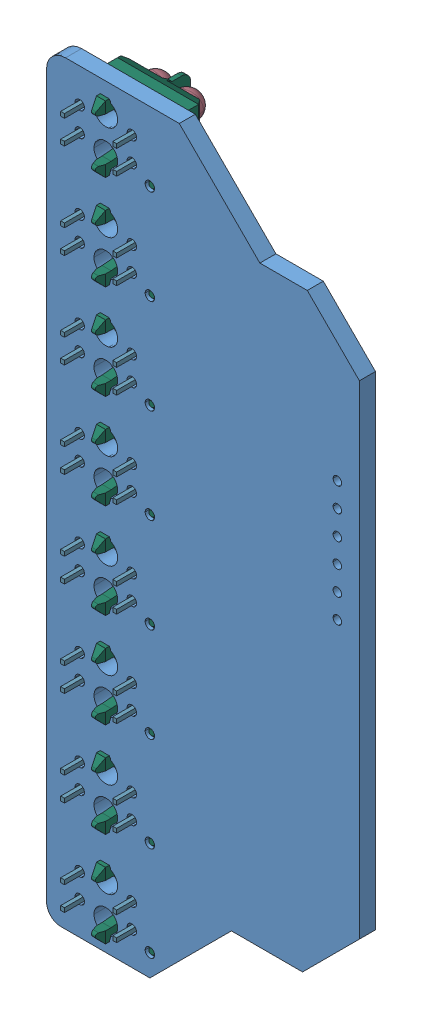
SolidWorks assembly Linelance_PCB v1.1, configuration По умолчанию. Lengths in mm. (continued)
Components (placement in the parent): (continued)
- Linelance_PCB v1.1.step-1: Linelance_PCB v1.1.step [По умолчанию] at origin size (33 79.6 10.52) (continued)
  - Linelance_PCB v1.1.step.step-1: Linelance_PCB v1.1.step.step [По умолчанию] at origin size (33 79.6 10.52) (continued)
    - R8.step.step-1: R8.step.step [По умолчанию] at origin size (0.8 1.6 0.5) (continued)
      - 5770190160.step-6.step-1: 5770190160.step-6.step [По умолчанию] at (4.2 69.8 -1.692) x (0 -1 0) z (0 0 -1) size (1.6 0.8 0.5)
        - Terminal-2.step-12.step-1: Terminal-2.step-12.step [По умолчанию] at (-0.8 -0.4 0) size (0.3 0.8 0.5)
          - Open_CASCADE_STEP_translator_6.8_7.2.1-6.step.step-1: Open_CASCADE_STEP_translator_6.8_7.2.1-6.step.step [По умолчанию] at origin size (0.3 0.8 0.5)
        - Terminal-2.step-13.step-1: Terminal-2.step-13.step [По умолчанию] at (0.8 0.4 0) x (-1 0 0) z (0 0 1) size (0.3 0.8 0.5)
          - Open_CASCADE_STEP_translator_6.8_7.2.1-6.step.step-1: Open_CASCADE_STEP_translator_6.8_7.2.1-6.step.step [По умолчанию] at origin size (0.3 0.8 0.5)
        - Mid_Body-7.step.step-1: Mid_Body-7.step.step [По умолчанию] at (-0.8 -0.4 0) size (1.5 0.8 0.4)
        - Mark-8.step.step-1: Mark-8.step.step [По умолчанию] at (-0.5 -0.4 0.45) size (1 0.8 0.05)
    - R7.step.step-1: R7.step.step [По умолчанию] at origin size (1.6 0.8 0.5)
      - 5770196880.step-1.step-1: 5770196880.step-1.step [По умолчанию] at (20.1975 53.1275 -1.692) x (-1 0 0) z (0 0 -1) size (1.6 0.8 0.5)
        - Terminal.step-2.step-1: Terminal.step-2.step [По умолчанию] at (-0.8 -0.4 0) size (0.3 0.8 0.5)
          - Open_CASCADE_STEP_translator_6.8_7.2.1.step.step-1: Open_CASCADE_STEP_translator_6.8_7.2.1.step.step [По умолчанию] at origin size (0.3 0.8 0.5)
        - Terminal.step-3.step-1: Terminal.step-3.step [По умолчанию] at (0.8 0.4 0) x (-1 0 0) z (0 0 1) size (0.3 0.8 0.5)
          - Open_CASCADE_STEP_translator_6.8_7.2.1.step.step-1: Open_CASCADE_STEP_translator_6.8_7.2.1.step.step [По умолчанию] at origin size (0.3 0.8 0.5)
        - Mid_Body.step.step-1: Mid_Body.step.step [По умолчанию] at (-0.8 -0.4 0) size (1.5 0.8 0.4)
        - Mark.step.step-1: Mark.step.step [По умолчанию] at (-0.5 -0.4 0.45) size (1 0.8 0.05)
    - R6.step.step-1: R6.step.step [По умолчанию] at origin size (1.6 0.8 0.5)
      - 5770190480.step.step-1: 5770190480.step.step [По умолчанию] at (20.9975 51.7275 -1.692) x (1 0 0) z (0 0 -1) size (1.6 0.8 0.5)
        - Terminal-3.step.step-1: Terminal-3.step.step [По умолчанию] at (-0.8 -0.4 0) size (0.3 0.8 0.5)
          - Open_CASCADE_STEP_translator_6.8_7.2.1-9.step.step-1: Open_CASCADE_STEP_translator_6.8_7.2.1-9.step.step [По умолчанию] at origin size (0.3 0.8 0.5)
        - Terminal-3.step-1.step-1: Terminal-3.step-1.step [По умолчанию] at (0.8 0.4 0) x (-1 0 0) z (0 0 1) size (0.3 0.8 0.5)
          - Open_CASCADE_STEP_translator_6.8_7.2.1-9.step.step-1: Open_CASCADE_STEP_translator_6.8_7.2.1-9.step.step [По умолчанию] at origin size (0.3 0.8 0.5)
        - Mid_Body-10.step.step-1: Mid_Body-10.step.step [По умолчанию] at (-0.8 -0.4 0) size (1.5 0.8 0.4)
        - Mark-11.step.step-1: Mark-11.step.step [По умолчанию] at (-0.5 -0.4 0.45) size (1 0.8 0.05)
    - R3.step.step-1: R3.step.step [По умолчанию] at origin size (0.8 1.6 0.5)
      - 5770190160.step-7.step-1: 5770190160.step-7.step [По умолчанию] at (18.5 26.9 -1.692) x (0 -1 0) z (0 0 -1) size (1.6 0.8 0.5)
        - Terminal-2.step-14.step-1: Terminal-2.step-14.step [По умолчанию] at (-0.8 -0.4 0) size (0.3 0.8 0.5)
          - Open_CASCADE_STEP_translator_6.8_7.2.1-6.step.step-1: Open_CASCADE_STEP_translator_6.8_7.2.1-6.step.step [По умолчанию] at origin size (0.3 0.8 0.5)
        - Terminal-2.step-15.step-1: Terminal-2.step-15.step [По умолчанию] at (0.8 0.4 0) x (-1 0 0) z (0 0 1) size (0.3 0.8 0.5)
          - Open_CASCADE_STEP_translator_6.8_7.2.1-6.step.step-1: Open_CASCADE_STEP_translator_6.8_7.2.1-6.step.step [По умолчанию] at origin size (0.3 0.8 0.5)
        - Mid_Body-7.step.step-1: Mid_Body-7.step.step [По умолчанию] at (-0.8 -0.4 0) size (1.5 0.8 0.4)
        - Mark-8.step.step-1: Mark-8.step.step [По умолчанию] at (-0.5 -0.4 0.45) size (1 0.8 0.05)
    - R2.step.step-1: R2.step.step [По умолчанию] at origin size (1.6 0.8 0.5)
      - 5770190480.step-1.step-1: 5770190480.step-1.step [По умолчанию] at (26.5 22.6 -1.692) x (1 0 0) z (0 0 -1) size (1.6 0.8 0.5)
        - Terminal-3.step-2.step-1: Terminal-3.step-2.step [По умолчанию] at (-0.8 -0.4 0) size (0.3 0.8 0.5)
          - Open_CASCADE_STEP_translator_6.8_7.2.1-9.step.step-1: Open_CASCADE_STEP_translator_6.8_7.2.1-9.step.step [По умолчанию] at origin size (0.3 0.8 0.5)
        - Terminal-3.step-3.step-1: Terminal-3.step-3.step [По умолчанию] at (0.8 0.4 0) x (-1 0 0) z (0 0 1) size (0.3 0.8 0.5)
          - Open_CASCADE_STEP_translator_6.8_7.2.1-9.step.step-1: Open_CASCADE_STEP_translator_6.8_7.2.1-9.step.step [По умолчанию] at origin size (0.3 0.8 0.5)
        - Mid_Body-10.step.step-1: Mid_Body-10.step.step [По умолчанию] at (-0.8 -0.4 0) size (1.5 0.8 0.4)
        - Mark-11.step.step-1: Mark-11.step.step [По умолчанию] at (-0.5 -0.4 0.45) size (1 0.8 0.05)
    - R5.step.step-1: R5.step.step [По умолчанию] at origin size (1.6 0.8 0.5)
      - 5770190480.step-2.step-1: 5770190480.step-2.step [По умолчанию] at (30.3 39.9 -1.692) x (1 0 0) z (0 0 -1) size (1.6 0.8 0.5)
        - Terminal-3.step-4.step-1: Terminal-3.step-4.step [По умолчанию] at (-0.8 -0.4 0) size (0.3 0.8 0.5)
          - Open_CASCADE_STEP_translator_6.8_7.2.1-9.step.step-1: Open_CASCADE_STEP_translator_6.8_7.2.1-9.step.step [По умолчанию] at origin size (0.3 0.8 0.5)
        - Terminal-3.step-5.step-1: Terminal-3.step-5.step [По умолчанию] at (0.8 0.4 0) x (-1 0 0) z (0 0 1) size (0.3 0.8 0.5)
          - Open_CASCADE_STEP_translator_6.8_7.2.1-9.step.step-1: Open_CASCADE_STEP_translator_6.8_7.2.1-9.step.step [По умолчанию] at origin size (0.3 0.8 0.5)
        - Mid_Body-10.step.step-1: Mid_Body-10.step.step [По умолчанию] at (-0.8 -0.4 0) size (1.5 0.8 0.4)
        - Mark-11.step.step-1: Mark-11.step.step [По умолчанию] at (-0.5 -0.4 0.45) size (1 0.8 0.05)
    - R4.step.step-1: R4.step.step [По умолчанию] at origin size (1.6 0.8 0.5)
      - 5770190480.step-3.step-1: 5770190480.step-3.step [По умолчанию] at (30.3 38.5 -1.692) x (1 0 0) z (0 0 -1) size (1.6 0.8 0.5)
        - Terminal-3.step-6.step-1: Terminal-3.step-6.step [По умолчанию] at (-0.8 -0.4 0) size (0.3 0.8 0.5)
          - Open_CASCADE_STEP_translator_6.8_7.2.1-9.step.step-1: Open_CASCADE_STEP_translator_6.8_7.2.1-9.step.step [По умолчанию] at origin size (0.3 0.8 0.5)
        - Terminal-3.step-7.step-1: Terminal-3.step-7.step [По умолчанию] at (0.8 0.4 0) x (-1 0 0) z (0 0 1) size (0.3 0.8 0.5)
          - Open_CASCADE_STEP_translator_6.8_7.2.1-9.step.step-1: Open_CASCADE_STEP_translator_6.8_7.2.1-9.step.step [По умолчанию] at origin size (0.3 0.8 0.5)
        - Mid_Body-10.step.step-1: Mid_Body-10.step.step [По умолчанию] at (-0.8 -0.4 0) size (1.5 0.8 0.4)
        - Mark-11.step.step-1: Mark-11.step.step [По умолчанию] at (-0.5 -0.4 0.45) size (1 0.8 0.05)
    - L4.step.step-1: L4.step.step [По умолчанию] at origin size (3.2 1.6 1.8)
      - 5770190080.step.step-1: 5770190080.step.step [По умолчанию] at (19.2675 55.0275 -1.692) x (-1 0 0) z (0 0 -1) size (3.2 1.6 1.8)
        - Terminal-4.step.step-1: Terminal-4.step.step [По умолчанию] at (-1.6 -0.8 0) size (3.2 1.6 1.8)
          - Open_CASCADE_STEP_translator_6.8_9.1.1.step.step-1: Open_CASCADE_STEP_translator_6.8_9.1.1.step.step [По умолчанию] at origin size (0.7 1.6 1.8)
          - Open_CASCADE_STEP_translator_6.8_9.1.2.step.step-1: Open_CASCADE_STEP_translator_6.8_9.1.2.step.step [По умолчанию] at origin size (0.7 1.6 1.8)
        - Mid_Body-12.step.step-1: Mid_Body-12.step.step [По умолчанию] at (-1.6 -0.8 0) size (1.8 1.6 1.8)
          - Open_CASCADE_STEP_translator_6.8_9.2.1.step.step-1: Open_CASCADE_STEP_translator_6.8_9.2.1.step.step [По умолчанию] at origin size (1.8 1.6 1.8)
    - L3.step.step-1: L3.step.step [По умолчанию] at origin size (1.6 3.2 1.8)
      - 5770196320.step.step-1: 5770196320.step.step [По умолчанию] at (19 40.5 -1.692) x (0 -1 0) z (0 0 -1) size (3.2 1.6 1.8)
        - Terminal-5.step.step-1: Terminal-5.step.step [По умолчанию] at (-1.6 -0.8 0) size (3.2 1.6 1.8)
          - Open_CASCADE_STEP_translator_6.8_9.1.1-13.step.step-1: Open_CASCADE_STEP_translator_6.8_9.1.1-13.step.step [По умолчанию] at origin size (0.7 1.6 1.8)
          - Open_CASCADE_STEP_translator_6.8_9.1.2-14.step.step-1: Open_CASCADE_STEP_translator_6.8_9.1.2-14.step.step [По умолчанию] at origin size (0.7 1.6 1.8)
        - Mid_Body-1.step.step-1: Mid_Body-1.step.step [По умолчанию] at (-1.6 -0.8 0) size (1.8 1.6 1.8)
          - Open_CASCADE_STEP_translator_6.8_9.2.1-15.step.step-1: Open_CASCADE_STEP_translator_6.8_9.2.1-15.step.step [По умолчанию] at origin size (1.8 1.6 1.8)
    - L2.step.step-1: L2.step.step [По умолчанию] at origin size (1.6 3.2 1.8)
      - 5770196320.step-1.step-1: 5770196320.step-1.step [По умолчанию] at (21.2975 44.5275 -1.692) x (0 -1 0) z (0 0 -1) size (3.2 1.6 1.8)
        - Terminal-5.step-1.step-1: Terminal-5.step-1.step [По умолчанию] at (-1.6 -0.8 0) size (3.2 1.6 1.8)
          - Open_CASCADE_STEP_translator_6.8_9.1.1-13.step.step-1: Open_CASCADE_STEP_translator_6.8_9.1.1-13.step.step [По умолчанию] at origin size (0.7 1.6 1.8)
          - Open_CASCADE_STEP_translator_6.8_9.1.2-14.step.step-1: Open_CASCADE_STEP_translator_6.8_9.1.2-14.step.step [По умолчанию] at origin size (0.7 1.6 1.8)
        - Mid_Body-1.step-1.step-1: Mid_Body-1.step-1.step [По умолчанию] at (-1.6 -0.8 0) size (1.8 1.6 1.8)
          - Open_CASCADE_STEP_translator_6.8_9.2.1-15.step.step-1: Open_CASCADE_STEP_translator_6.8_9.2.1-15.step.step [По умолчанию] at origin size (1.8 1.6 1.8)
    - L1.step.step-1: L1.step.step [По умолчанию] at origin size (3.2 1.6 1.8)
      - 5770190080.step-1.step-1: 5770190080.step-1.step [По умолчанию] at (24.1 57.3 -1.692) x (-1 0 0) z (0 0 -1) size (3.2 1.6 1.8)
        - Terminal-4.step-1.step-1: Terminal-4.step-1.step [По умолчанию] at (-1.6 -0.8 0) size (3.2 1.6 1.8)
          - Open_CASCADE_STEP_translator_6.8_9.1.1.step.step-1: Open_CASCADE_STEP_translator_6.8_9.1.1.step.step [По умолчанию] at origin size (0.7 1.6 1.8)
          - Open_CASCADE_STEP_translator_6.8_9.1.2.step.step-1: Open_CASCADE_STEP_translator_6.8_9.1.2.step.step [По умолчанию] at origin size (0.7 1.6 1.8)
        - Mid_Body-12.step-1.step-1: Mid_Body-12.step-1.step [По умолчанию] at (-1.6 -0.8 0) size (1.8 1.6 1.8)
          - Open_CASCADE_STEP_translator_6.8_9.2.1.step.step-1: Open_CASCADE_STEP_translator_6.8_9.2.1.step.step [По умолчанию] at origin size (1.8 1.6 1.8)
    - D1.step.step-1: D1.step.step [По умолчанию] at origin size (1.7 0.9 0.7)
      - SOD523.step.step-1: SOD523.step.step [По умолчанию] at (30.4001 58.3999 -1.692) x (1 0 0) z (0 0 -1) size (1.7 0.9 0.7)
    - C21.step.step-1: C21.step.step [По умолчанию] at origin size (0.8 1.6 0.5)
      - 5899457520.step-1.step-1: 5899457520.step-1.step [По умолчанию] at (17.9975 52.3525 -2.192) size (0.8 1 0.5)
        - Extruded-1.step.step-1: Extruded-1.step.step [По умолчанию] at origin size (0.8 1 0.5)
      - 5899457200.step-2.step-1: 5899457200.step-2.step [По умолчанию] at (17.9975 53.0025 -2.192) size (0.8 0.3 0.5)
        - Extruded-2.step.step-1: Extruded-2.step.step [По умолчанию] at origin size (0.8 0.3 0.5)
      - 5899457200.step-3.step-1: 5899457200.step-3.step [По умолчанию] at (17.9975 51.7025 -2.192) size (0.8 0.3 0.5)
        - Extruded-2.step.step-1: Extruded-2.step.step [По умолчанию] at origin size (0.8 0.3 0.5)
    - C20.step.step-1: C20.step.step [По умолчанию] at origin size (0.8 1.6 0.5)
      - 5899457200.step-4.step-1: 5899457200.step-4.step [По умолчанию] at (17.9975 49.9775 -2.192) size (0.8 0.3 0.5)
        - Extruded-2.step.step-1: Extruded-2.step.step [По умолчанию] at origin size (0.8 0.3 0.5)
      - 5899457200.step-5.step-1: 5899457200.step-5.step [По умолчанию] at (17.9975 48.6775 -2.192) size (0.8 0.3 0.5)
        - Extruded-2.step.step-1: Extruded-2.step.step [По умолчанию] at origin size (0.8 0.3 0.5)
      - 5899457520.step-2.step-1: 5899457520.step-2.step [По умолчанию] at (17.9975 49.3275 -2.192) size (0.8 1 0.5)
        - Extruded-1.step.step-1: Extruded-1.step.step [По умолчанию] at origin size (0.8 1 0.5)
    - C14.step.step-1: C14.step.step [По умолчанию] at origin size (1.6 0.8 0.5)
      - 5899458880.step-4.step-1: 5899458880.step-4.step [По умолчанию] at (18.6 36.1 -2.192) size (1 0.8 0.5)
        - Extruded.step.step-1: Extruded.step.step [По умолчанию] at origin size (1 0.8 0.5)
      - 5899458400.step-8.step-1: 5899458400.step-8.step [По умолчанию] at (19.25 36.1 -2.192) size (0.3 0.8 0.5)
        - Extruded-0.step.step-1: Extruded-0.step.step [По умолчанию] at origin size (0.3 0.8 0.5)
      - 5899458400.step-9.step-1: 5899458400.step-9.step [По умолчанию] at (17.95 36.1 -2.192) size (0.3 0.8 0.5)
        - Extruded-0.step.step-1: Extruded-0.step.step [По умолчанию] at origin size (0.3 0.8 0.5)
    - C13.step.step-1: C13.step.step [По умолчанию] at origin size (1.6 0.8 0.5)
      - 5899458880.step-5.step-1: 5899458880.step-5.step [По умолчанию] at (18.6 37.4 -2.192) size (1 0.8 0.5)
        - Extruded.step.step-1: Extruded.step.step [По умолчанию] at origin size (1 0.8 0.5)
      - 5899458400.step-10.step-1: 5899458400.step-10.step [По умолчанию] at (19.25 37.4 -2.192) size (0.3 0.8 0.5)
        - Extruded-0.step.step-1: Extruded-0.step.step [По умолчанию] at origin size (0.3 0.8 0.5)
      - 5899458400.step-11.step-1: 5899458400.step-11.step [По умолчанию] at (17.95 37.4 -2.192) size (0.3 0.8 0.5)
        - Extruded-0.step.step-1: Extruded-0.step.step [По умолчанию] at origin size (0.3 0.8 0.5)
    - C9.step.step-1: C9.step.step [По умолчанию] at origin size (0.8 1.6 0.5)
      - 5899457520.step-3.step-1: 5899457520.step-3.step [По умолчанию] at (23.2 43.7 -2.192) size (0.8 1 0.5)
        - Extruded-1.step.step-1: Extruded-1.step.step [По умолчанию] at origin size (0.8 1 0.5)
      - 5899457200.step-6.step-1: 5899457200.step-6.step [По умолчанию] at (23.2 43.05 -2.192) size (0.8 0.3 0.5)
        - Extruded-2.step.step-1: Extruded-2.step.step [По умолчанию] at origin size (0.8 0.3 0.5)
      - 5899457200.step-7.step-1: 5899457200.step-7.step [По умолчанию] at (23.2 44.35 -2.192) size (0.8 0.3 0.5)
        - Extruded-2.step.step-1: Extruded-2.step.step [По умолчанию] at origin size (0.8 0.3 0.5)
    - C10.step.step-1: C10.step.step [По умолчанию] at origin size (0.8 1.6 0.5)
      - 5899457520.step-4.step-1: 5899457520.step-4.step [По умолчанию] at (24.7 43.7 -2.192) size (0.8 1 0.5)
        - Extruded-1.step.step-1: Extruded-1.step.step [По умолчанию] at origin size (0.8 1 0.5)
      - 5899457200.step-8.step-1: 5899457200.step-8.step [По умолчанию] at (24.7 43.05 -2.192) size (0.8 0.3 0.5)
        - Extruded-2.step.step-1: Extruded-2.step.step [По умолчанию] at origin size (0.8 0.3 0.5)
      - 5899457200.step-9.step-1: 5899457200.step-9.step [По умолчанию] at (24.7 44.35 -2.192) size (0.8 0.3 0.5)
        - Extruded-2.step.step-1: Extruded-2.step.step [По умолчанию] at origin size (0.8 0.3 0.5)
    - C12.step.step-1: C12.step.step [По умолчанию] at origin size (0.8 1.6 0.5)
      - 5899457520.step-5.step-1: 5899457520.step-5.step [По умолчанию] at (27.6968 43.7 -2.192) size (0.8 1 0.5)
        - Extruded-1.step.step-1: Extruded-1.step.step [По умолчанию] at origin size (0.8 1 0.5)
      - 5899457200.step-10.step-1: 5899457200.step-10.step [По умолчанию] at (27.6968 43.05 -2.192) size (0.8 0.3 0.5)
        - Extruded-2.step.step-1: Extruded-2.step.step [По умолчанию] at origin size (0.8 0.3 0.5)
      - 5899457200.step-11.step-1: 5899457200.step-11.step [По умолчанию] at (27.6968 44.35 -2.192) size (0.8 0.3 0.5)
        - Extruded-2.step.step-1: Extruded-2.step.step [По умолчанию] at origin size (0.8 0.3 0.5)
    - C19.step.step-1: C19.step.step [По умолчанию] at origin size (0.8 1.6 0.5)
      - 5899457520.step-6.step-1: 5899457520.step-6.step [По умолчанию] at (20 25.7 -2.192) size (0.8 1 0.5)
        - Extruded-1.step.step-1: Extruded-1.step.step [По умолчанию] at origin size (0.8 1 0.5)
      - 5899457200.step-12.step-1: 5899457200.step-12.step [По умолчанию] at (20 26.35 -2.192) size (0.8 0.3 0.5)
        - Extruded-2.step.step-1: Extruded-2.step.step [По умолчанию] at origin size (0.8 0.3 0.5)
      - 5899457200.step-13.step-1: 5899457200.step-13.step [По умолчанию] at (20 25.05 -2.192) size (0.8 0.3 0.5)
        - Extruded-2.step.step-1: Extruded-2.step.step [По умолчанию] at origin size (0.8 0.3 0.5)
    - C18.step.step-1: C18.step.step [По умолчанию] at origin size (1.6 0.8 0.5)
      - 5899458880.step-6.step-1: 5899458880.step-6.step [По умолчанию] at (25.3 32.2 -2.192) size (1 0.8 0.5)
        - Extruded.step.step-1: Extruded.step.step [По умолчанию] at origin size (1 0.8 0.5)
      - 5899458400.step-12.step-1: 5899458400.step-12.step [По умолчанию] at (25.95 32.2 -2.192) size (0.3 0.8 0.5)
        - Extruded-0.step.step-1: Extruded-0.step.step [По умолчанию] at origin size (0.3 0.8 0.5)
      - 5899458400.step-13.step-1: 5899458400.step-13.step [По умолчанию] at (24.65 32.2 -2.192) size (0.3 0.8 0.5)
        - Extruded-0.step.step-1: Extruded-0.step.step [По умолчанию] at origin size (0.3 0.8 0.5)
    - C17.step.step-1: C17.step.step [По умолчанию] at origin size (1.6 0.8 0.5)
      - 5899458880.step-7.step-1: 5899458880.step-7.step [По умолчанию] at (23.3 33.7 -2.192) size (1 0.8 0.5)
        - Extruded.step.step-1: Extruded.step.step [По умолчанию] at origin size (1 0.8 0.5)
      - 5899458400.step-14.step-1: 5899458400.step-14.step [По умолчанию] at (22.65 33.7 -2.192) size (0.3 0.8 0.5)
        - Extruded-0.step.step-1: Extruded-0.step.step [По умолчанию] at origin size (0.3 0.8 0.5)
      - 5899458400.step-15.step-1: 5899458400.step-15.step [По умолчанию] at (23.95 33.7 -2.192) size (0.3 0.8 0.5)
        - Extruded-0.step.step-1: Extruded-0.step.step [По умолчанию] at origin size (0.3 0.8 0.5)
    - C5.step.step-1: C5.step.step [По умолчанию] at origin size (0.8 1.6 0.5)
      - 5899457520.step-7.step-1: 5899457520.step-7.step [По умолчанию] at (27.7 46.7 -2.192) size (0.8 1 0.5)
        - Extruded-1.step.step-1: Extruded-1.step.step [По умолчанию] at origin size (0.8 1 0.5)
      - 5899457200.step-14.step-1: 5899457200.step-14.step [По умолчанию] at (27.7 47.35 -2.192) size (0.8 0.3 0.5)
        - Extruded-2.step.step-1: Extruded-2.step.step [По умолчанию] at origin size (0.8 0.3 0.5)
      - 5899457200.step-15.step-1: 5899457200.step-15.step [По умолчанию] at (27.7 46.05 -2.192) size (0.8 0.3 0.5)
        - Extruded-2.step.step-1: Extruded-2.step.step [По умолчанию] at origin size (0.8 0.3 0.5)
    - C8.step.step-1: C8.step.step [По умолчанию] at origin size (0.8 1.6 0.5)
      - 5899457520.step-8.step-1: 5899457520.step-8.step [По умолчанию] at (23.2 46.7 -2.192) size (0.8 1 0.5)
        - Extruded-1.step.step-1: Extruded-1.step.step [По умолчанию] at origin size (0.8 1 0.5)
      - 5899457200.step-16.step-1: 5899457200.step-16.step [По умолчанию] at (23.2 46.05 -2.192) size (0.8 0.3 0.5)
        - Extruded-2.step.step-1: Extruded-2.step.step [По умолчанию] at origin size (0.8 0.3 0.5)
      - 5899457200.step-17.step-1: 5899457200.step-17.step [По умолчанию] at (23.2 47.35 -2.192) size (0.8 0.3 0.5)
        - Extruded-2.step.step-1: Extruded-2.step.step [По умолчанию] at origin size (0.8 0.3 0.5)
    - C7.step.step-1: C7.step.step [По умолчанию] at origin size (0.8 1.6 0.5)
      - 5899457520.step-9.step-1: 5899457520.step-9.step [По умолчанию] at (24.7 46.7 -2.192) size (0.8 1 0.5)
        - Extruded-1.step.step-1: Extruded-1.step.step [По умолчанию] at origin size (0.8 1 0.5)
      - 5899457200.step-18.step-1: 5899457200.step-18.step [По умолчанию] at (24.7 46.05 -2.192) size (0.8 0.3 0.5)
        - Extruded-2.step.step-1: Extruded-2.step.step [По умолчанию] at origin size (0.8 0.3 0.5)
      - 5899457200.step-19.step-1: 5899457200.step-19.step [По умолчанию] at (24.7 47.35 -2.192) size (0.8 0.3 0.5)
        - Extruded-2.step.step-1: Extruded-2.step.step [По умолчанию] at origin size (0.8 0.3 0.5)
    - C6.step.step-1: C6.step.step [По умолчанию] at origin size (0.8 1.6 0.5)
      - 5899457520.step-10.step-1: 5899457520.step-10.step [По умолчанию] at (26.2 46.7 -2.192) size (0.8 1 0.5)
        - Extruded-1.step.step-1: Extruded-1.step.step [По умолчанию] at origin size (0.8 1 0.5)
      - 5899457200.step-20.step-1: 5899457200.step-20.step [По умолчанию] at (26.2 46.05 -2.192) size (0.8 0.3 0.5)
        - Extruded-2.step.step-1: Extruded-2.step.step [По умолчанию] at origin size (0.8 0.3 0.5)
      - 5899457200.step-21.step-1: 5899457200.step-21.step [По умолчанию] at (26.2 47.35 -2.192) size (0.8 0.3 0.5)
        - Extruded-2.step.step-1: Extruded-2.step.step [По умолчанию] at origin size (0.8 0.3 0.5)
    - C3.step.step-1: C3.step.step [По умолчанию] at origin size (0.8 1.6 0.5)
      - 5899457520.step-11.step-1: 5899457520.step-11.step [По умолчанию] at (23 54.6573 -2.192) size (0.8 1 0.5)
        - Extruded-1.step.step-1: Extruded-1.step.step [По умолчанию] at origin size (0.8 1 0.5)
      - 5899457200.step-22.step-1: 5899457200.step-22.step [По умолчанию] at (23 54.0073 -2.192) size (0.8 0.3 0.5)
        - Extruded-2.step.step-1: Extruded-2.step.step [По умолчанию] at origin size (0.8 0.3 0.5)
      - 5899457200.step-23.step-1: 5899457200.step-23.step [По умолчанию] at (23 55.3073 -2.192) size (0.8 0.3 0.5)
        - Extruded-2.step.step-1: Extruded-2.step.step [По умолчанию] at origin size (0.8 0.3 0.5)
    - C2.step.step-1: C2.step.step [По умолчанию] at origin size (0.8 1.6 0.5)
      - 5899457520.step-12.step-1: 5899457520.step-12.step [По умолчанию] at (25.7 54.6573 -2.192) size (0.8 1 0.5)
        - Extruded-1.step.step-1: Extruded-1.step.step [По умолчанию] at origin size (0.8 1 0.5)
      - 5899457200.step-24.step-1: 5899457200.step-24.step [По умолчанию] at (25.7 55.3073 -2.192) size (0.8 0.3 0.5)
        - Extruded-2.step.step-1: Extruded-2.step.step [По умолчанию] at origin size (0.8 0.3 0.5)
      - 5899457200.step-25.step-1: 5899457200.step-25.step [По умолчанию] at (25.7 54.0073 -2.192) size (0.8 0.3 0.5)
        - Extruded-2.step.step-1: Extruded-2.step.step [По умолчанию] at origin size (0.8 0.3 0.5)
